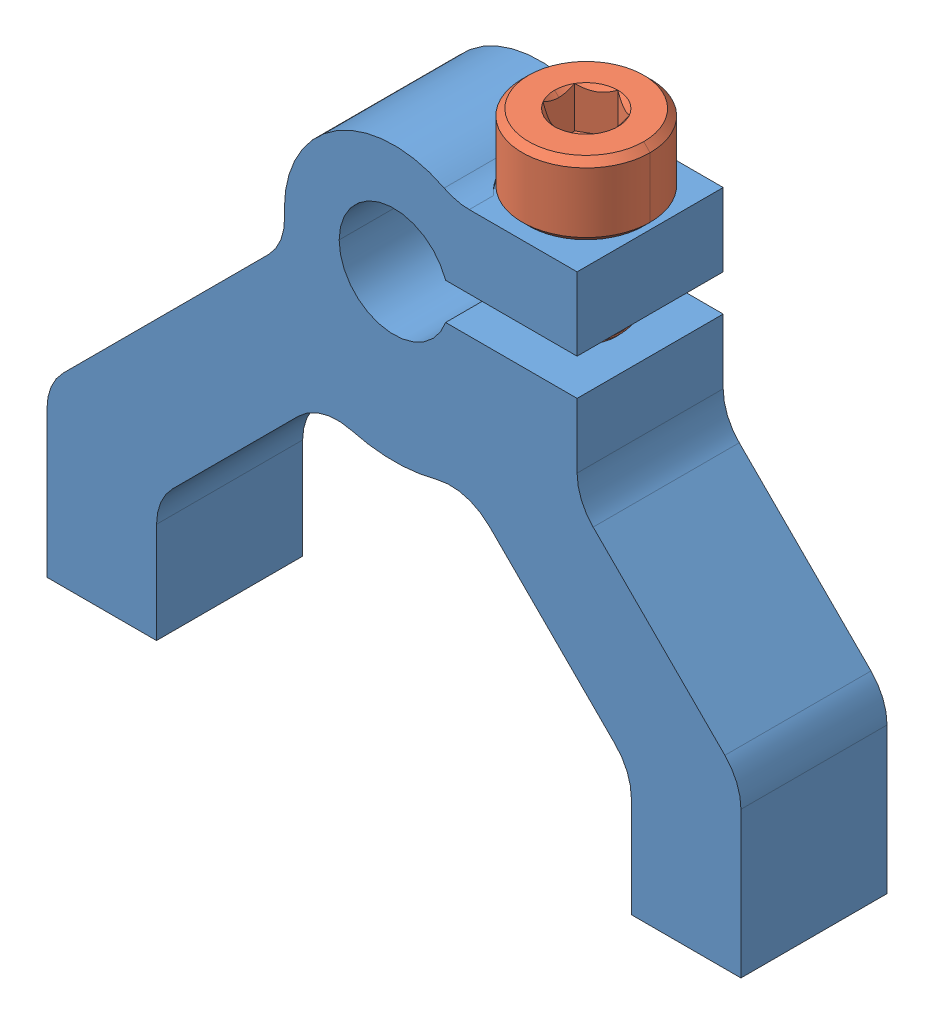
SolidWorks assembly 1400-0032-0006 assembly, configuration Default. Lengths in mm.
Overall size (38 33.01 8).
3 component instances, 2 part files, 0 mates.
Components (placement in the parent):
- 1400-0032-0006 assembly.STEP-1: 1400-0032-0006 assembly.STEP [Default] at origin size (38 33.01 8)
  - 1400-0032-0006.STEP-1: 1400-0032-0006.STEP [Default] at (-10.4545 5.2733 4.1329) size (38 30 8)
  - 2800-0004-0010_90128A207.STEP-1: 2800-0004-0010_90128A207.STEP [Default] at (-3.9261 0.2733 8.1329) x (1 0 0) z (0 -1 0) size (7 7 14.01)
